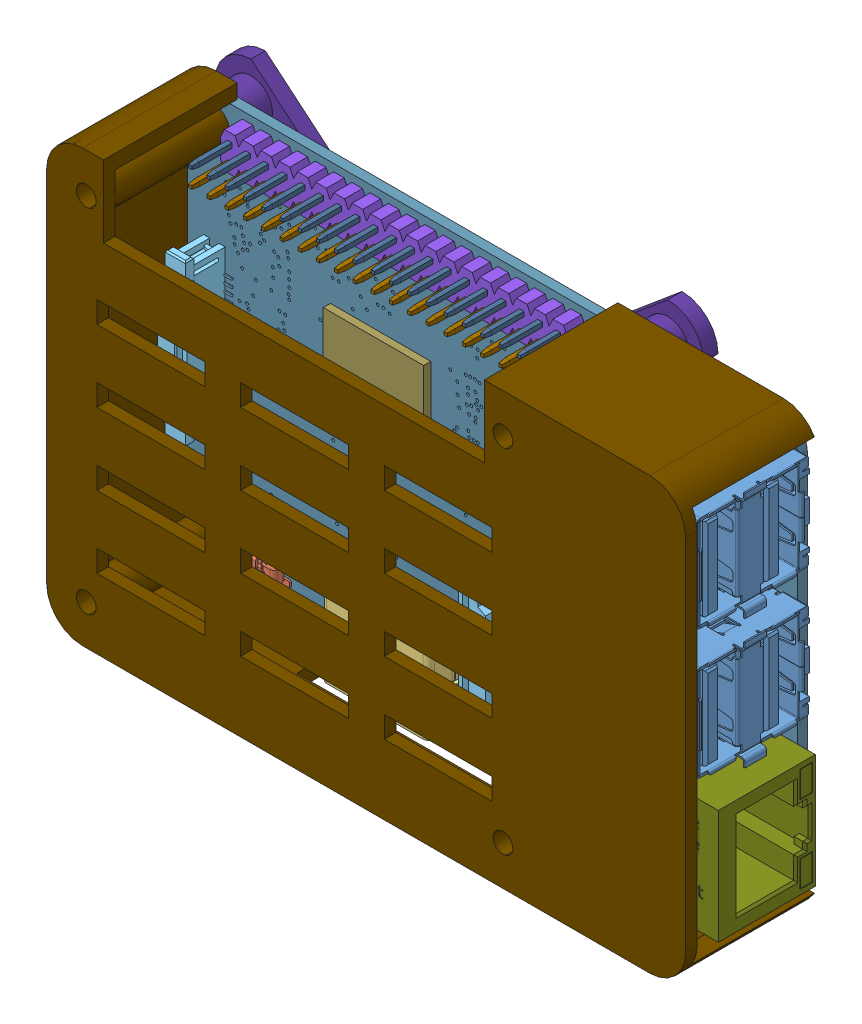
SolidWorks assembly ulemine elektroonika, configuration Default. Lengths in mm.
Overall size (89.64 60 24.93).
61 component instances, 18 part files, 6 mates.
Components (placement in the parent):
- Raspberry pi 3 cad model-1: Raspberry pi 3 cad model [Default] at origin size (89.64 57.31 18.59)
  - raspberrypi_3_stripped.step-1: raspberrypi_3_stripped.step [Default] at origin size (89.64 57.31 18.59)
    - RPi3_ModelB v1.step-1: RPi3_ModelB v1.step [Default] at (-6 -61 0) x (1 0 0) z (0 -1 0) size (86.09 18.24 56.14)
      - MOLEX_672983090.step-1: MOLEX_672983090.step [Default] at (30.19 0.8 -64.5) x (0 0 -1) z (1 0 0) size (15.47 17.24 17.92)
      - MOLEX_672983090.step-2: MOLEX_672983090.step [Default] at (30.19 0.8 -82.5) x (0 0 -1) z (1 0 0) size (15.47 17.24 17.92)
      - molex_0473460001.step-1: molex_0473460001.step [Default] at (-31.9 0.8 -37.765) size (7.98 2.76 5.43)
      - molex_0471510001.step-1: molex_0471510001.step [Default] at (-10.5 0.65 -34.125) size (15.04 7.63 12.15)
      - PJ-322.step-1: PJ-322.step [Default] at (11.1 0.8 -42.85) size (7.23 7.55 15)
      - te_1-1734248-5.step-1: te_1-1734248-5.step [Default] at (-38.7109 0.8 -63.5) x (0 0 1) z (-1 0 0) size (22.4 5.68 5.07)
      - te_1-1734248-5.step-2: te_1-1734248-5.step [Default] at (2.058 0.82 -46.9107) x (0 0 -1) z (1 0 0) size (22.4 5.68 5.07)
      - MOLEX_1040310811.step-1: MOLEX_1040310811.step [Default] at (-35.065 -0.3 -63.58) x (0 0 -1) z (-1 0 0) size (11.95 1.45 11.4)
      - raspberry_pi_3(RJ45).step-1: raspberry_pi_3(RJ45).step [Default] at (44.6723 16.4551 -37.9773) x (0 0 -1) z (1 0 0) size (9.5 2.68 12.61)
    - Raspberry Pi 3157.step-1: Raspberry Pi 3157.step [Default] at origin size (50.8 5 2.5)
    - Raspberry Pi 3242.step-1: Raspberry Pi 3242.step [Default] at (0.3 0 0) size (0.64 0.64 5.5)
    - Raspberry Pi 3266.step-1: Raspberry Pi 3266.step [Default] at (0.3 -0.1777 0) size (0.64 0.64 5.5)
    - raspberry_pi_3(bar_180_2x20).step-1: raspberry_pi_3(bar_180_2x20).step [Default] at (-40.3908 28.1775 3.5) x (0 1 0) z (-1 0 0) size (3.19 3.1 48.91)
    - Raspberry Pi 312.step-1: Raspberry Pi 312.step [Default] at origin size (13.97 14.11 1)
    - Raspberry Pi 3180.step-1: Raspberry Pi 3180.step [Default] at origin size (0.5 0.3 0.3)
    - Raspberry Pi 31.step-1: Raspberry Pi 31.step [Default] at origin size (84.92 56 1.33)
    - raspberry_pi_B+_(microsd2).step-1: raspberry_pi_B+_(microsd2).step [Default] at (-43.2065 2.73 -0.97) x (1 0 0) z (0 1 0) size (15 0.97 11)
    - Raspberry Pi 3242.step-2: Raspberry Pi 3242.step [Default] at (2.84 0 0) size (0.64 0.64 5.5)
    - Raspberry Pi 3242.step-3: Raspberry Pi 3242.step [Default] at (5.38 0 0) size (0.64 0.64 5.5)
    - Raspberry Pi 3242.step-4: Raspberry Pi 3242.step [Default] at (7.92 0 0) size (0.64 0.64 5.5)
    - Raspberry Pi 3242.step-5: Raspberry Pi 3242.step [Default] at (10.46 0 0) size (0.64 0.64 5.5)
    - Raspberry Pi 3242.step-6: Raspberry Pi 3242.step [Default] at (13 0 0) size (0.64 0.64 5.5)
    - Raspberry Pi 3242.step-7: Raspberry Pi 3242.step [Default] at (15.54 0 0) size (0.64 0.64 5.5)
    - Raspberry Pi 3242.step-8: Raspberry Pi 3242.step [Default] at (18.08 0 0) size (0.64 0.64 5.5)
    - Raspberry Pi 3242.step-9: Raspberry Pi 3242.step [Default] at (20.62 0 0) size (0.64 0.64 5.5)
    - Raspberry Pi 3242.step-10: Raspberry Pi 3242.step [Default] at (23.16 0 0) size (0.64 0.64 5.5)
    - Raspberry Pi 3242.step-11: Raspberry Pi 3242.step [Default] at (25.7 0 0) size (0.64 0.64 5.5)
    - Raspberry Pi 3242.step-12: Raspberry Pi 3242.step [Default] at (28.24 0 0) size (0.64 0.64 5.5)
    - Raspberry Pi 3242.step-13: Raspberry Pi 3242.step [Default] at (30.78 0 0) size (0.64 0.64 5.5)
    - Raspberry Pi 3242.step-14: Raspberry Pi 3242.step [Default] at (33.32 0 0) size (0.64 0.64 5.5)
    - Raspberry Pi 3242.step-15: Raspberry Pi 3242.step [Default] at (35.86 0 0) size (0.64 0.64 5.5)
    - Raspberry Pi 3242.step-16: Raspberry Pi 3242.step [Default] at (38.4 0 0) size (0.64 0.64 5.5)
    - Raspberry Pi 3242.step-17: Raspberry Pi 3242.step [Default] at (40.94 0 0) size (0.64 0.64 5.5)
    - Raspberry Pi 3242.step-18: Raspberry Pi 3242.step [Default] at (43.48 0 0) size (0.64 0.64 5.5)
    - Raspberry Pi 3242.step-19: Raspberry Pi 3242.step [Default] at (46.02 0 0) size (0.64 0.64 5.5)
    - Raspberry Pi 3242.step-20: Raspberry Pi 3242.step [Default] at (48.56 0 0) size (0.64 0.64 5.5)
    - Raspberry Pi 3266.step-2: Raspberry Pi 3266.step [Default] at (2.84 -0.1777 0) size (0.64 0.64 5.5)
    - Raspberry Pi 3266.step-3: Raspberry Pi 3266.step [Default] at (5.38 -0.1777 0) size (0.64 0.64 5.5)
    - Raspberry Pi 3266.step-4: Raspberry Pi 3266.step [Default] at (7.92 -0.1777 0) size (0.64 0.64 5.5)
    - Raspberry Pi 3266.step-5: Raspberry Pi 3266.step [Default] at (10.46 -0.1777 0) size (0.64 0.64 5.5)
    - Raspberry Pi 3266.step-6: Raspberry Pi 3266.step [Default] at (13 -0.1777 0) size (0.64 0.64 5.5)
    - Raspberry Pi 3266.step-7: Raspberry Pi 3266.step [Default] at (15.54 -0.1777 0) size (0.64 0.64 5.5)
    - Raspberry Pi 3266.step-8: Raspberry Pi 3266.step [Default] at (18.08 -0.1777 0) size (0.64 0.64 5.5)
    - Raspberry Pi 3266.step-9: Raspberry Pi 3266.step [Default] at (20.62 -0.1777 0) size (0.64 0.64 5.5)
    - Raspberry Pi 3266.step-10: Raspberry Pi 3266.step [Default] at (23.16 -0.1777 0) size (0.64 0.64 5.5)
    - Raspberry Pi 3266.step-11: Raspberry Pi 3266.step [Default] at (25.7 -0.1777 0) size (0.64 0.64 5.5)
    - Raspberry Pi 3266.step-12: Raspberry Pi 3266.step [Default] at (28.24 -0.1777 0) size (0.64 0.64 5.5)
    - Raspberry Pi 3266.step-13: Raspberry Pi 3266.step [Default] at (30.78 -0.1777 0) size (0.64 0.64 5.5)
    - Raspberry Pi 3266.step-14: Raspberry Pi 3266.step [Default] at (33.32 -0.1777 0) size (0.64 0.64 5.5)
    - Raspberry Pi 3266.step-15: Raspberry Pi 3266.step [Default] at (35.86 -0.1777 0) size (0.64 0.64 5.5)
    - Raspberry Pi 3266.step-16: Raspberry Pi 3266.step [Default] at (38.4 -0.1777 0) size (0.64 0.64 5.5)
    - Raspberry Pi 3266.step-17: Raspberry Pi 3266.step [Default] at (40.94 -0.1777 0) size (0.64 0.64 5.5)
    - Raspberry Pi 3266.step-18: Raspberry Pi 3266.step [Default] at (43.48 -0.1777 0) size (0.64 0.64 5.5)
    - Raspberry Pi 3266.step-19: Raspberry Pi 3266.step [Default] at (46.02 -0.1777 0) size (0.64 0.64 5.5)
    - Raspberry Pi 3266.step-20: Raspberry Pi 3266.step [Default] at (48.56 -0.1777 0) size (0.64 0.64 5.5)
    - raspberry_pi_B_(RJ45).step-1: raspberry_pi_B_(RJ45).step [Default] at (38.93 -23.19 14.5) x (0 1 0) z (1 0 0) size (15.88 16.5 21.4)
- Raspberry kinnitus v1.1-1: Raspberry kinnitus v1.1 [Default] at (18.058 -27.0893 -6.33) x (0 1 0) z (1 0 0) size (59 6 68)
- rasberry kate-1: rasberry kate [Default] at (-5.7203 -11.4652 17) x (0 1 0) z (1 0 0) size (60 18.6 88.93)
Mates (geometry in assembly coordinates):
- Concentric1: concentric anti-aligned: cylinder of Raspberry pi 3 cad model-1/raspberrypi_3_stripped.step-1/Raspberry Pi 31.step-1 through (13.058 26.9107 -0.75) axis (0 0 1) radius 1.375; cylinder of Raspberry kinnitus v1.1-1 through (13.058 26.9107 -4.33) axis (0 0 -1) radius 1
- Concentric2: concentric anti-aligned: cylinder of Raspberry pi 3 cad model-1/raspberrypi_3_stripped.step-1/Raspberry Pi 31.step-1 through (13.058 -22.0893 -0.75) axis (0 0 1) radius 1.375; cylinder of Raspberry kinnitus v1.1-1 through (13.058 -22.0893 -4.33) axis (0 0 -1) radius 1
- Coincident1: coincident anti-aligned: plane of Raspberry pi 3 cad model-1/raspberrypi_3_stripped.step-1/Raspberry Pi 31.step-1 through (36.4822 30.4107 -0.33) normal (0 0 -1); plane of Raspberry kinnitus v1.1-1 through (13.058 26.9107 -0.33) normal (0 0 1)
- Concentric5: concentric anti-aligned: cylinder of Raspberry pi 3 cad model-1/raspberrypi_3_stripped.step-1/Raspberry Pi 31.step-1 through (-44.942 26.9107 -0.75) axis (0 0 1) radius 1.375; cylinder of rasberry kate-1 through (-44.942 26.9107 18.6) axis (0 0 -1) radius 1.375
- Concentric6: concentric aligned: cylinder of Raspberry kinnitus v1.1-1 through (13.058 26.9107 -0.33) axis (0 0 -1) radius 3; cylinder of rasberry kate-1 through (13.058 26.9107 18.6) axis (0 0 -1) radius 1.375
- Coincident3: coincident anti-aligned: plane of Raspberry pi 3 cad model-1/raspberrypi_3_stripped.step-1/Raspberry Pi 31.step-1 through (-48.452 -25.5993 1) normal (0 0 1); plane of rasberry kate-1 through (-44.942 26.9107 1) normal (0 0 -1)
